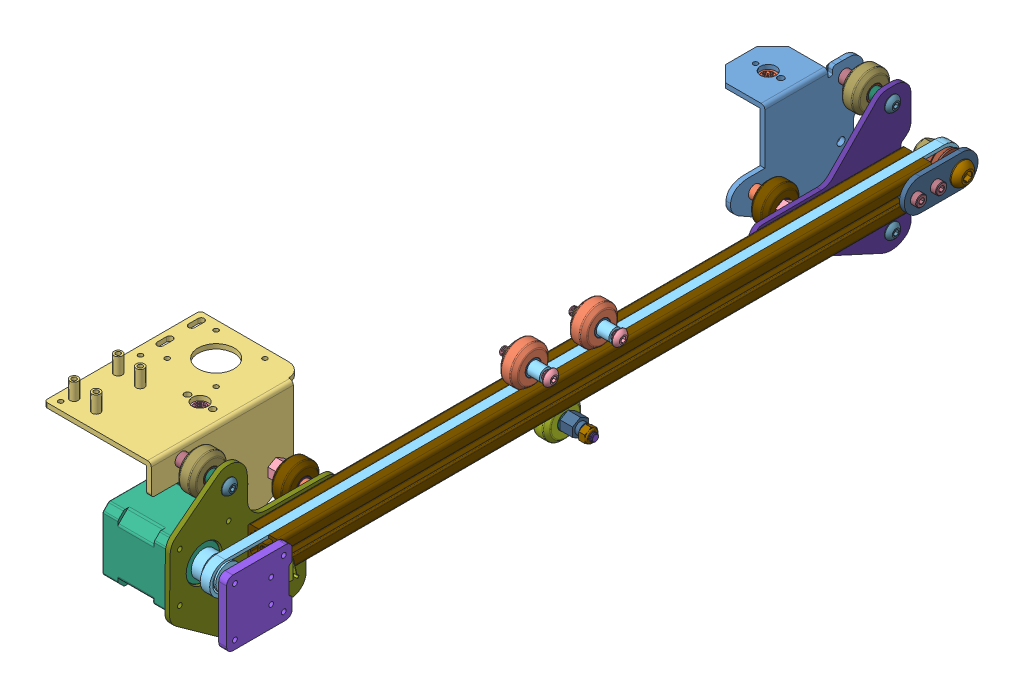
SolidWorks assembly CR10 v1.step, configuration Default. Lengths in mm.
Overall size (136.73 100.1 489.87).
99 component instances, 43 part files, 0 mates.
Components (placement in the parent):
- CR-10S Pro Assembly.step-1: CR-10S Pro Assembly.step [Default] at origin size (136.73 100.1 489.87)
  - Z Axis.step-1: Z Axis.step [Default] at (0 250 0) size (136.73 100.1 489.87)
    - X.step-1: X.step [Default] at (0 0 -50) size (47.15 64.01 68)
      - Wheel Kit - X.step-1: Wheel Kit - X.step [Default] at origin size (37.34 24 24)
        - Roller Wheel, Bearing v4 (13) (1) (1).step-1: Roller Wheel, Bearing v4 (13) (1) (1).step [Default] at (0 0 -104.5247) x (1 0 0) z (0 1 0) size (11 24 24)
          - 6153K69 (1) (1).step-1: 6153K69 (1) (1).step [Default] at (199.5253 -7.1977 167.0806) x (0 -1 0) z (1 0 0) size (16 16 11)
          - Wheel (1) (1).step-1: Wheel (1) (1).step [Default] at (199.5253 -7.1977 167.0806) x (0 -1 0) z (1 0 0) size (24 24 11)
        - 94645A102 (1) (1) (1).step-1: 94645A102 (1) (1) (1).step [Default] at (194.0253 167.0806 -97.327) x (0 0 1) z (0 -1 0) size (8 5.01 9.24)
        - 92095A218 (1) (1) (1).step-1: 92095A218 (1) (1) (1).step [Default] at (218.3253 167.0806 -97.327) x (0 0 1) z (1 0 0) size (12.44 10.38 37.34)
        - 92871A045 (2) (1) (1).step-1: 92871A045 (2) (1) (1).step [Default] at (209.0253 167.0806 -97.327) x (0 0 1) z (1 0 0) size (8 8 8)
      - Wheel Kit - X (1).step-1: Wheel Kit - X (1).step [Default] at (0 -0.0178 -44) size (37.34 24 24)
        - Roller Wheel, Bearing v4 (13) (1) (1) (1).step-1: Roller Wheel, Bearing v4 (13) (1) (1) (1).step [Default] at (0 0 -104.5247) x (1 0 0) z (0 1 0) size (11 24 24)
          - 6153K69 (1) (1).step-1: 6153K69 (1) (1).step [Default] at (199.5253 -7.1977 167.0806) x (0 -1 0) z (1 0 0) size (16 16 11)
          - Wheel (1) (1).step-1: Wheel (1) (1).step [Default] at (199.5253 -7.1977 167.0806) x (0 -1 0) z (1 0 0) size (24 24 11)
        - 94645A102 (1) (1) (1).step-1: 94645A102 (1) (1) (1).step [Default] at (194.0253 167.0806 -97.327) x (0 0 1) z (0 -1 0) size (8 5.01 9.24)
        - 92095A218 (1) (1) (1).step-1: 92095A218 (1) (1) (1).step [Default] at (218.3253 167.0806 -97.327) x (0 0 1) z (1 0 0) size (12.44 10.38 37.34)
        - 92871A045 (2) (1) (1).step-1: 92871A045 (2) (1) (1).step [Default] at (209.0253 167.0806 -97.327) x (0 0 1) z (1 0 0) size (8 8 8)
      - Wheel Kit - X Hex.step-1: Wheel Kit - X Hex.step [Default] at (0 1.4879 -2) size (37.34 24 24)
        - Roller Wheel, Bearing v4 (12) (1) (1).step-1: Roller Wheel, Bearing v4 (12) (1) (1).step [Default] at (0 0 -79.2271) x (1 0 0) z (0 1 0) size (11 24 24)
          - 6153K69 (1) (2).step-1: 6153K69 (1) (2).step [Default] at (199.0453 37.1 125.5806) x (0 -1 0) z (1 0 0) size (16 16 11)
          - Wheel (1) (2).step-1: Wheel (1) (2).step [Default] at (199.0453 37.1 125.5806) x (0 -1 0) z (1 0 0) size (24 24 11)
        - 92095A218 (1) (1) (2).step-1: 92095A218 (1) (1) (2).step [Default] at (190.7953 125.5806 -116.327) x (0 0 1) z (-1 0 0) size (12.44 10.38 37.34)
        - 94645A102 (1) (1) (2).step-1: 94645A102 (1) (1) (2).step [Default] at (216.7253 125.5806 -116.327) x (0 0 1) z (0 1 0) size (8 5.01 9.24)
        - Hex Nut, Eccentric v2 (1) (1).step-1: Hex Nut, Eccentric v2 (1) (1).step [Default] at (205.1253 125.5806 -117.327) x (0 0 1) z (1 0 0) size (10 11.55 11.08)
      - X Carriage.step-1: X Carriage.step [Default] at (213.0253 -220.3918 24.765) x (0 0 1) z (0 1 0) (suppressed, hidden)
    - Wheel Kit - Y Left.step-1: Wheel Kit - Y Left.step [Default] at origin size (45.15 24 24)
      - Roller Wheel, Bearing v4 (7) (1).step-1: Roller Wheel, Bearing v4 (7) (1).step [Default] at (0 0 89.3615) size (11 24 24)
        - 6153K69 (1).step-1: 6153K69 (1).step [Default] at (172.9025 182.9944 -58.9807) x (0 0 1) z (-1 0 0) size (16 16 11)
        - Wheel (1).step-1: Wheel (1).step [Default] at (172.9025 182.9944 -58.9807) x (0 0 1) z (-1 0 0) size (24 24 11)
      - 92871A045 (1) (1).step-1: 92871A045 (1) (1).step [Default] at (163.4025 182.9944 30.3808) x (0 0 1) z (1 0 0) size (8 8 8)
      - 94500A302 (1).step-1: 94500A302 (1).step [Default] at (192.1525 182.9944 30.3808) x (0 0 1) z (1 0 0) size (11.15 11.15 45.15)
      - 92871A045 (1) (2).step-1: 92871A045 (1) (2).step [Default] at (182.4025 182.9944 30.3808) x (0 0 1) z (1 0 0) size (8 8 8)
      - 94645A102 (2) (1).step-1: 94645A102 (2) (1).step [Default] at (156.4025 182.9944 30.3808) x (0 0 -1) z (0 1 0) size (8 5.01 9.24)
    - Wheel Kit - Y Left (1).step-1: Wheel Kit - Y Left (1).step [Default] at (0 -70.0486 0) size (45.15 24 24)
      - Roller Wheel, Bearing v4 (7) (1) (1).step-1: Roller Wheel, Bearing v4 (7) (1) (1).step [Default] at (0 0 89.3615) size (11 24 24)
        - 6153K69 (1).step-1: 6153K69 (1).step [Default] at (172.9025 182.9944 -58.9807) x (0 0 1) z (-1 0 0) size (16 16 11)
        - Wheel (1).step-1: Wheel (1).step [Default] at (172.9025 182.9944 -58.9807) x (0 0 1) z (-1 0 0) size (24 24 11)
      - 92871A045 (1) (1).step-1: 92871A045 (1) (1).step [Default] at (163.4025 182.9944 30.3808) x (0 0 1) z (1 0 0) size (8 8 8)
      - 94500A302 (1).step-1: 94500A302 (1).step [Default] at (192.1525 182.9944 30.3808) x (0 0 1) z (1 0 0) size (11.15 11.15 45.15)
      - 92871A045 (1) (2).step-1: 92871A045 (1) (2).step [Default] at (182.4025 182.9944 30.3808) x (0 0 1) z (1 0 0) size (8 8 8)
      - 94645A102 (2) (1).step-1: 94645A102 (2) (1).step [Default] at (156.4025 182.9944 30.3808) x (0 0 -1) z (0 1 0) size (8 5.01 9.24)
    - Wheel Kit - Y Left Hex.step-1: Wheel Kit - Y Left Hex.step [Default] at (0 -34.8875 -58.9744) size (45.15 24 24)
      - Roller Wheel, Bearing v4 (7) (1) (1) (1).step-1: Roller Wheel, Bearing v4 (7) (1) (1) (1).step [Default] at (0 0 89.3615) size (11 24 24)
        - 6153K69 (1) (3).step-1: 6153K69 (1) (3).step [Default] at (172.9025 182.9944 -58.9807) x (0 0 1) z (-1 0 0) size (16 16 11)
        - Wheel (1) (3).step-1: Wheel (1) (3).step [Default] at (172.9025 182.9944 -58.9807) x (0 0 1) z (-1 0 0) size (24 24 11)
      - 94500A302 (1) (1).step-1: 94500A302 (1) (1).step [Default] at (192.1525 182.9944 30.3808) x (0 0 1) z (1 0 0) size (11.15 11.15 45.15)
      - 92871A045 (1) (2) (1).step-1: 92871A045 (1) (2) (1).step [Default] at (182.4025 182.9944 30.3808) x (0 0 1) z (1 0 0) size (8 8 8)
      - 94645A102 (2) (1) (1).step-1: 94645A102 (2) (1) (1).step [Default] at (156.4025 182.9944 30.3808) x (0 0 -1) z (0 1 0) size (8 5.01 9.24)
      - Hex Nut, Eccentric v2 (1).step-1: Hex Nut, Eccentric v2 (1).step [Default] at (166.8225 182.9944 29.3808) x (0 0 1) z (-1 0 0) size (10 11.55 11.08)
    - Nema17.step-1: Nema17.step [Default] at (145.9025 148.3914 45.8889) x (0 0 -1) z (0 -1 0) size (42 64 48.25)
      - GT20-20-5(Mirror) (1) (1).step-1: GT20-20-5(Mirror) (1) (1).step [Default] at (0 42.8 0) x (0 1 0) z (1 0 0) size (16 16 16)
      - Nema17-0.step-1: Nema17-0.step [Default] at origin size (42 64 48.25)
    - X-Axis Endstop Switch Plate v3 (1).step-1: X-Axis Endstop Switch Plate v3 (1).step [Default] at (219.4025 146.9944 45.8808) x (1 0 0) z (0 1 0) size (12 52.4 41.6)
      - Lerdge microswitch v2 (1) (1) (1).step-1: Lerdge microswitch v2 (1) (1) (1).step [Default] at (-7 11.5 0) x (0 0 1) z (1 0 0) size (22 29.6 6.9)
      - X-Axis Endstop Switch Plate v3 (1)-1.step-1: X-Axis Endstop Switch Plate v3 (1)-1.step [Default] at origin size (5 41.6 41.6)
    - X Idle (1).step-1: X Idle (1).step [Default] x (1 0 0) z (0 1 0) size (29.45 46.8 20.2)
      - 91306A679 (1).step-1: 91306A679 (1).step [Default] at (217.1083 411.2715 145.9944) x (0 -1 0) z (1 0 0) size (14 14 29.4)
      - X-Axis, Bracket, Tension, Pulley v2 (1).step-1: X-Axis, Bracket, Tension, Pulley v2 (1).step [Default] at (209.6583 385.2715 146.9944) x (0 1 0) z (0 0 -1) size (46.8 3.05 20.2)
      - 7804K147 (1).step-1: 7804K147 (1).step [Default] at (203.1583 411.2715 145.9944) x (0 -1 0) z (-1 0 0) size (18 18 5)
      - 7804K147 (1).step-2: 7804K147 (1).step [Default] at (198.1583 411.2715 145.9944) x (0 -1 0) z (1 0 0) size (18 18 5)
      - 90576A117 (1).step-1: 90576A117 (1).step [Default] at (195.6583 411.2715 145.9944) x (0 -1 0) z (0 0 -1) size (13 8.02 15.01)
      - 91292A108 (1) (1).step-1: 91292A108 (1) (1).step [Default] at (204.3583 395.2715 146.9944) x (0 -1 0) z (-1 0 0) size (7 7 12)
      - 91292A108 (1) (1).step-2: 91292A108 (1) (1).step [Default] at (204.7083 382.2715 146.9944) x (0 -1 0) z (-1 0 0) size (7 7 12)
      - M4, T-Slot Nut v1 (1).step-1: M4, T-Slot Nut v1 (1).step [Default] at (203.9583 382.2715 146.9944) x (0 0 -1) z (0 -1 0) size (11.5 5.74 6.24)
      - M4, T-Slot Nut v1 (1).step-2: M4, T-Slot Nut v1 (1).step [Default] at (203.9583 395.2715 146.9944) x (0 0 -1) z (0 -1 0) size (11.5 5.74 6.24)
      - 90710A120 (1).step-1: 90710A120 (1).step [Default] at (207.6583 411.2715 145.9944) x (0 -1 0) z (0 0 1) size (13 4.01 15.01)
    - Wheel Kit - Y Left (2).step-1: Wheel Kit - Y Left (2).step [Default] at (0 0 -421) size (45.15 24 24)
      - Roller Wheel, Bearing v4 (7) (1) (2).step-1: Roller Wheel, Bearing v4 (7) (1) (2).step [Default] at (0 0 89.3615) size (11 24 24)
        - 6153K69 (1).step-1: 6153K69 (1).step [Default] at (172.9025 182.9944 -58.9807) x (0 0 1) z (-1 0 0) size (16 16 11)
        - Wheel (1).step-1: Wheel (1).step [Default] at (172.9025 182.9944 -58.9807) x (0 0 1) z (-1 0 0) size (24 24 11)
      - 92871A045 (1) (1).step-1: 92871A045 (1) (1).step [Default] at (163.4025 182.9944 30.3808) x (0 0 1) z (1 0 0) size (8 8 8)
      - 94500A302 (1).step-1: 94500A302 (1).step [Default] at (192.1525 182.9944 30.3808) x (0 0 1) z (1 0 0) size (11.15 11.15 45.15)
      - 92871A045 (1) (2).step-1: 92871A045 (1) (2).step [Default] at (182.4025 182.9944 30.3808) x (0 0 1) z (1 0 0) size (8 8 8)
      - 94645A102 (2) (1).step-1: 94645A102 (2) (1).step [Default] at (156.4025 182.9944 30.3808) x (0 0 -1) z (0 1 0) size (8 5.01 9.24)
    - Wheel Kit - Y Left (3).step-1: Wheel Kit - Y Left (3).step [Default] at (0 -69.9484 -421) size (45.15 24 24)
      - Roller Wheel, Bearing v4 (7) (1) (3).step-1: Roller Wheel, Bearing v4 (7) (1) (3).step [Default] at (0 0 89.3615) size (11 24 24)
        - 6153K69 (1).step-1: 6153K69 (1).step [Default] at (172.9025 182.9944 -58.9807) x (0 0 1) z (-1 0 0) size (16 16 11)
        - Wheel (1).step-1: Wheel (1).step [Default] at (172.9025 182.9944 -58.9807) x (0 0 1) z (-1 0 0) size (24 24 11)
      - 92871A045 (1) (1).step-1: 92871A045 (1) (1).step [Default] at (163.4025 182.9944 30.3808) x (0 0 1) z (1 0 0) size (8 8 8)
      - 94500A302 (1).step-1: 94500A302 (1).step [Default] at (192.1525 182.9944 30.3808) x (0 0 1) z (1 0 0) size (11.15 11.15 45.15)
      - 92871A045 (1) (2).step-1: 92871A045 (1) (2).step [Default] at (182.4025 182.9944 30.3808) x (0 0 1) z (1 0 0) size (8 8 8)
      - 94645A102 (2) (1).step-1: 94645A102 (2) (1).step [Default] at (156.4025 182.9944 30.3808) x (0 0 -1) z (0 1 0) size (8 5.01 9.24)
    - Wheel Kit - Y Left Hex (1).step-1: Wheel Kit - Y Left Hex (1).step [Default] at (345.3249 -34.9291 -303.2204) x (-1 0 0) z (0 0 -1) size (45.15 24 24)
      - Roller Wheel, Bearing v4 (7) (1) (1) (2).step-1: Roller Wheel, Bearing v4 (7) (1) (1) (2).step [Default] at (0 0 89.3615) size (11 24 24)
        - 6153K69 (1) (3).step-1: 6153K69 (1) (3).step [Default] at (172.9025 182.9944 -58.9807) x (0 0 1) z (-1 0 0) size (16 16 11)
        - Wheel (1) (3).step-1: Wheel (1) (3).step [Default] at (172.9025 182.9944 -58.9807) x (0 0 1) z (-1 0 0) size (24 24 11)
      - 94500A302 (1) (1).step-1: 94500A302 (1) (1).step [Default] at (192.1525 182.9944 30.3808) x (0 0 1) z (1 0 0) size (11.15 11.15 45.15)
      - 92871A045 (1) (2) (1).step-1: 92871A045 (1) (2) (1).step [Default] at (182.4025 182.9944 30.3808) x (0 0 1) z (1 0 0) size (8 8 8)
      - 94645A102 (2) (1) (1).step-1: 94645A102 (2) (1) (1).step [Default] at (156.4025 182.9944 30.3808) x (0 0 -1) z (0 1 0) size (8 5.01 9.24)
      - Hex Nut, Eccentric v2 (1).step-1: Hex Nut, Eccentric v2 (1).step [Default] at (166.8225 182.9944 29.3808) x (0 0 1) z (-1 0 0) size (10 11.55 11.08)
    - Z Axis Front Left.step-1: Z Axis Front Left.step [Default] at (186.4025 515.7025 79.4868) x (0 0 -1) z (0 -1 0) size (108.21 3 93.17)
    - Z Axis Front Right.step-1: Z Axis Front Right.step [Default] at (186.4025 514.8685 -171.377) x (0 0 -1) z (0 -1 0) size (101.38 3 89.79)
    - 5537T751 (1).step-1: 5537T751 (1).step [Default] at (199.5304 146.9944 18.3808) x (0 0 1) z (0 1 0) size (415 19.99 19.99)
    - Z Axis Back Right.step-1: Z Axis Back Right.step [Default] at (159.4025 409.8685 -171.377) x (0 0 -1) z (0 -1 0) size (85.25 35 89.77)
    - Nut, Flange, M8 v2 (1).step-1: Nut, Flange, M8 v2 (1).step [Default] at (141.4025 189.3421 -360.1192) x (0 0 1) z (0 1 0) size (12.5 22 9.1)
    - Z Axis Back Left.step-1: Z Axis Back Left.step [Default] at (156.4025 283.5951 187.3974) x (0 0 -1) z (0 -1 0) size (99.16 70 99.48)
    - Nut, Flange, M8 v2 (2) (1).step-1: Nut, Flange, M8 v2 (2) (1).step [Default] at (141.4025 187.4944 0) x (0 0 1) z (0 1 0) size (12.5 22 9.1)
    - X-Axis Belt_CR-10S v1 (1).step-1: X-Axis Belt_CR-10S v1 (1).step [Default] at (196.8285 146.9946 45.8811) x (0 0 1) z (0 1 0) size (476.5 6 20)
    - Nema17 (1).step-1: Nema17 (1).step [Default] at (122.6118 146.9467 -28.4244) (suppressed, hidden)
